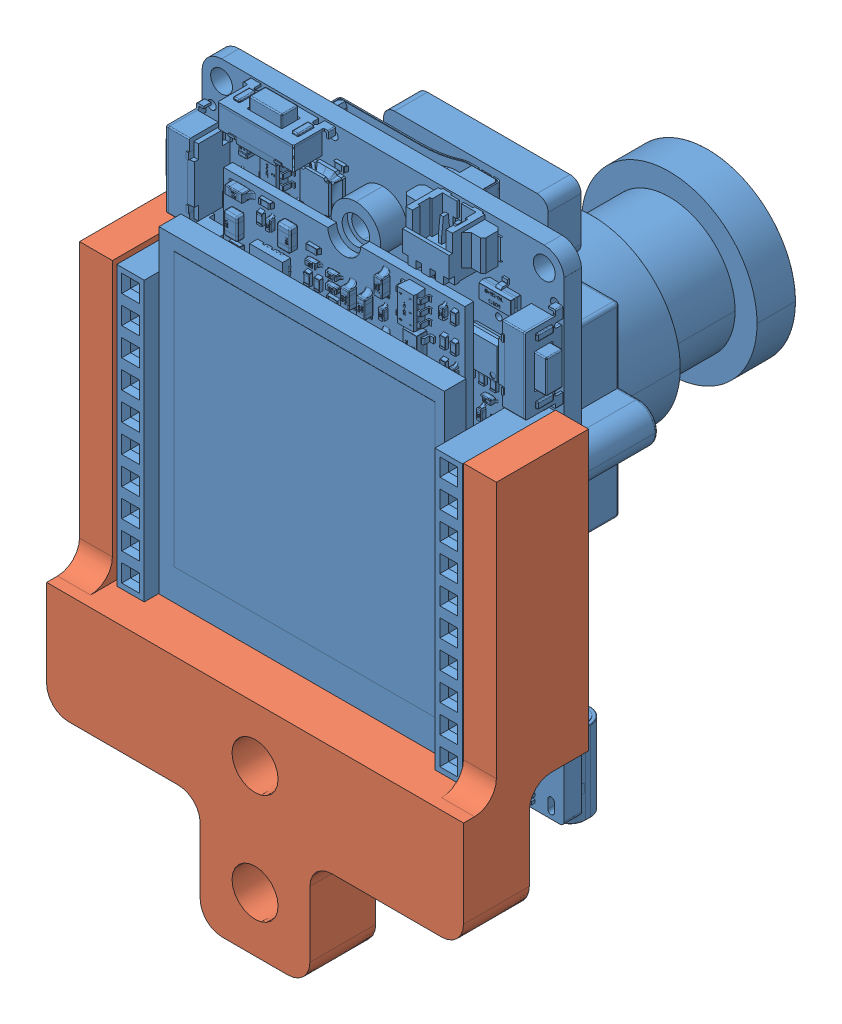
SolidWorks assembly 装配体230, configuration 默认. Lengths in mm.
Overall size (38 58.73 40.9).
2 component instances, 2 part files, 3 mates.
Components (placement in the parent):
- MAIX-DOCK-1: MAIX-DOCK [默认] at (-26.6435 4.8699 57.8676) size (34.73 47.37 38)
- DOCK支架-1: DOCK支架 [默认] at (-87.598 -61.3567 57.8676) x (0 -1 0) z (-1 0 0) size (45.4 11.4 38)
Mates (geometry in assembly coordinates):
- 重合1: coincident: plane of MAIX-DOCK-1 through (-10.9135 2.165 57.9676) normal (1 0 0); plane of DOCK支架-1 through (-10.9135 14.865 66.2676) normal (-1 0 0)
- 重合2: coincident: plane of MAIX-DOCK-1 through (-41.1635 14.865 66.3676) normal (0 1 0); plane of DOCK支架-1 through (-42.9135 14.865 66.2676) normal (0 1 0)
- 重合3: coincident anti-aligned: plane of MAIX-DOCK-1 through (-43.1465 -17.2391 57.8676) normal (0 0 1); plane of DOCK支架-1 through (-87.598 -61.3567 57.8676) normal (0 0 -1)
